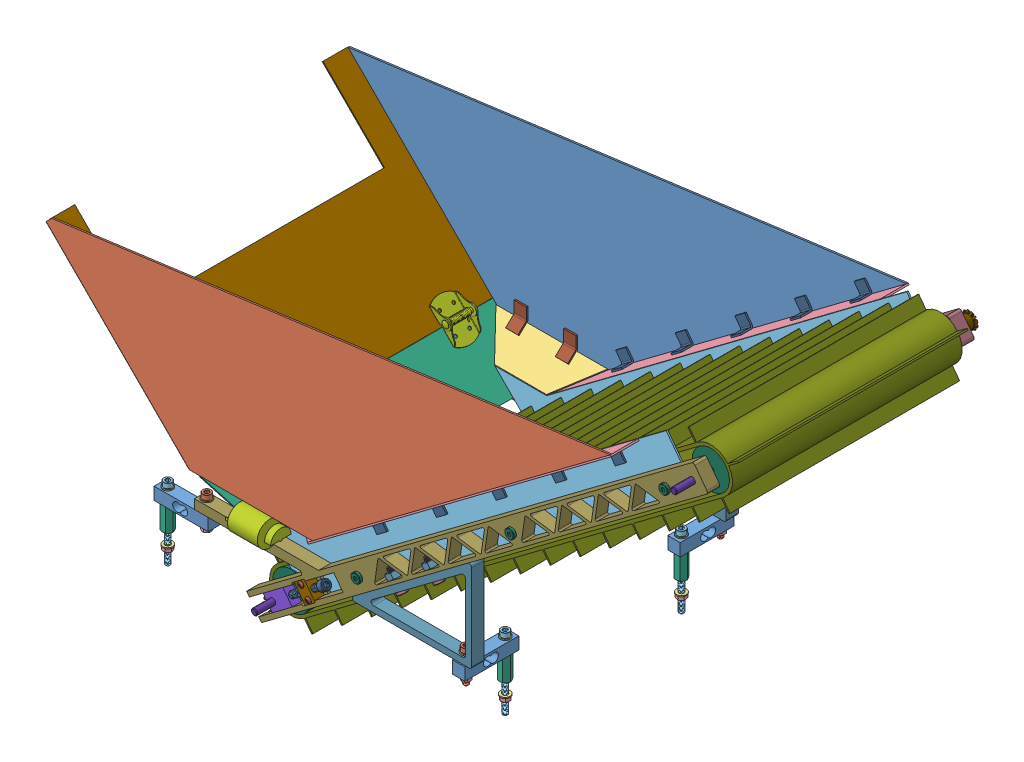
SolidWorks assembly Assembly_Hopper-Output, configuration Default. Lengths in mm.
Overall size (694.79 448.62 314.31).
124 component instances, 33 part files, 140 mates.
Components (placement in the parent):
- Side Plate Right-1: Side Plate Right [Default] at origin size (577.96 228.6 12.7)
- Side Plate Left-1: Side Plate Left [Default] at (0 0 303.2125) size (577.96 228.6 12.7)
- Slide-1: Slide [Default] at (0 1.1528 2.6789) x (1 0 0) z (0 -0.726184 -0.6875) size (114.3 38.1 1.59)
- Flap (Beside Conveyor)-4: Flap (Beside Conveyor) [Default] at (419.1 228.6 28.575) x (-0.8 -0.6 0) z (0.6 -0.8 0) size (425.45 28.57 1.59)
- Side Support-1: Side Support [Default] at (26.1937 -26.1937 28.575) size (451.96 314.33 1.59)
- Front Mesh 2-1: Front Mesh 2 [9227T543] at (20.048 -20.8922 152.4) x (0.707107 -0.707107 0) z (0 0 1) size (69.85 1.19 304.8)
- Front Hinge Bent-1: Front Hinge Bent [1613A11] at (-4.5491 4.5491 40.8686) x (0 0 -1) z (0.707107 -0.707107 0) size (30 12.7 42.82)
- Front Hinge Bent-4: Front Hinge Bent [1613A11] at (-7.2432 7.2432 264.7188) x (0 0 -1) z (0.707107 -0.707107 0) size (30 12.7 42.82)
- Front Folding Mesh-1: Front Folding Mesh [Default] at (-155.6871 149.5086 300.0375) x (-0.707107 -0.707107 0) z (0.707107 -0.707107 0) size (7.54 301.62 209.55)
  - Front Frame-1: Front Frame [Default] at origin size (6.35 301.62 209.55)
  - Front Mesh-1: Front Mesh [9227T543] at (-3.7719 147.6375 104.775) x (0 -1 0) z (0 0 1) size (301.62 1.19 209.55)
- Fastener-3: Fastener [Default] at (384.556 202.692 1.5875) x (0 0 1) z (-0.8 -0.6 0) size (12.7 12.7 12.7)
- Fastener-4: Fastener [Default] at (323.596 156.972 1.5875) x (0 0 1) z (-0.8 -0.6 0) size (12.7 12.7 12.7)
- Fastener-5: Fastener [Default] at (262.636 111.252 1.5875) x (0 0 1) z (-0.8 -0.6 0) size (12.7 12.7 12.7)
- Fastener-6: Fastener [Default] at (389.5725 204.47 28.575) x (0.6 -0.8 0) z (0.8 0.6 0) size (12.7 12.7 12.7)
- Fastener2-1: Fastener2 [Default] at (31.75 2.1861 1.5875) x (0 -0.6875 0.726184) z (-1 0 0) size (21.43 10.31 12.7)
- Fastener-7: Fastener [Default] at (328.6125 158.75 28.575) x (0.6 -0.8 0) z (0.8 0.6 0) size (12.7 12.7 12.7)
- Fastener-8: Fastener [Default] at (267.6525 113.03 28.575) x (0.6 -0.8 0) z (0.8 0.6 0) size (12.7 12.7 12.7)
- Fastener-10: Fastener [Default] at (374.396 195.072 303.2125) x (0 0 -1) z (0.8 0.6 0) size (12.7 12.7 12.7)
- Flap (Beside Conveyor)-5: Flap (Beside Conveyor) [Default] at (420.0525 227.33 276.225) x (-0.8 -0.6 0) z (-0.6 0.8 0) size (425.45 28.57 1.59)
- Fastener-13: Fastener [Default] at (313.436 149.352 303.2125) x (0 0 -1) z (0.8 0.6 0) size (12.7 12.7 12.7)
- Fastener-14: Fastener [Default] at (252.476 103.632 303.2125) x (0 0 -1) z (0.8 0.6 0) size (12.7 12.7 12.7)
- Slide-3: Slide [Default] at (0 0 303.2125) x (1 0 0) z (0 0.726184 -0.6875) size (114.3 38.1 1.59)
- Side Support-2: Side Support [Default] at (26.1937 -26.1937 274.6375) size (451.96 314.33 1.59)
- Fastener-16: Fastener [Default] at (399.7325 212.09 276.225) x (0.6 -0.8 0) z (-0.8 -0.6 0) size (12.7 12.7 12.7)
- Conveyor Beam Left-7: Conveyor Beam Left [Default] at (31.115 -94.1387 288.925) x (0.8 0.6 0) z (0 0 -1) size (586.74 101.6 12.7)
- Conveyor Beam Right-1: Conveyor Beam Right [Default] at (31.115 -94.1387 28.575) x (0.8 0.6 0) z (0 0 -1) size (586.74 101.6 12.7)
- Support-1: Support [Default] at (134.4083 -48.4188 276.225) size (121.92 92.72 12.7)
- Roller-1: Roller [Default] at (487.045 231.9338 34.925) x (-0.796427 -0.604735 0) z (0 0 1) size (38.1 38.1 234.95)
- Conveyor-1: Conveyor [Default] at (53.975 -116.6812 34.925) x (0.8 0.6 0) z (0 0 1) size (606.4 69.85 234.95)
- 12 inch shaft-1: 12 inch shaft [1257K66] at (487.045 231.9338 155.575) x (-0.158208 -0.987406 0) z (0 0 1) size (6.35 6.35 304.8)
- Gear2.0-1: Gear2.0 [6529K42] at (487.045 231.9338 15.0812) x (1 0 0) z (0 1 0) size (16.68 12.39 16.68)
- Roller-2: Roller [Default] at (57.785 -90.0113 269.875) x (0.803545 0.595244 0) z (0 0 -1) size (38.1 38.1 234.95)
- Fastener-17: Fastener [Default] at (338.7725 166.37 276.225) x (0.6 -0.8 0) z (-0.8 -0.6 0) size (12.7 12.7 12.7)
- Fastener-18: Fastener [Default] at (277.8125 120.65 276.225) x (0.6 -0.8 0) z (-0.8 -0.6 0) size (12.7 12.7 12.7)
- 12 inch shaft-2: 12 inch shaft [1257K66] at (57.785 -90.0113 155.575) x (0.992208 -0.124594 0) z (0 0 -1) size (6.35 6.35 304.8)
- Load_Cell_20_kg-1: Load_Cell_20_kg [Default] at (255.6933 -61.1187 290.195) x (0 0 -1) z (0 1 0) size (55.25 12.7 12.77)
- Load_Cell_20_kg-2: Load_Cell_20_kg [Default] at (242.9933 -61.1187 14.605) x (0 0 1) z (0 1 0) size (55.25 12.7 12.77)
- Load_Cell_20_kg-3: Load_Cell_20_kg [Default] at (-63.5 -61.1187 288.925) x (1 0 0) z (0 1 0) size (55.25 12.7 12.77)
- Load_Cell_20_kg-4: Load_Cell_20_kg [Default] at (-63.5 -61.1187 28.575) x (1 0 0) z (0 1 0) size (55.25 12.7 12.77)
- Screw for Load Cell M5x0.8x30mm-1: Screw for Load Cell M5x0.8x30mm [91290A194] at (-15.875 -50.2937 282.575) x (-0.988347 0 0.152214) z (0 1 0) size (8.5 8.5 35.43)
- Washer for Load Cell Screw-1: Washer for Load Cell Screw [93475A240] at (-15.875 -37.7938 282.575) x (1 0 0) z (0 -1 0) size (10 10 1.1)
- Washer for Load Cell Screw-2: Washer for Load Cell Screw [93475A240] at (-15.875 -62.2188 282.575) x (1 0 0) z (0 1 0) size (10 10 1.1)
- Nut for Load Cell Screw-2: Nut for Load Cell Screw [90592A095] at (-15.875 -64.2188 282.575) x (-0.979134 0 0.203217) z (-0.203217 0 -0.979134) size (8 4.62 9.24)
- Screw for Load Cell M5x0.8x30mm-2: Screw for Load Cell M5x0.8x30mm [91290A194] at (-15.875 -50.2937 22.225) x (-0.988347 0 -0.152214) z (0 1 0) size (8.5 8.5 35.43)
- Washer for Load Cell Screw-3: Washer for Load Cell Screw [93475A240] at (-15.875 -61.1187 22.225) x (1 0 0) z (0 -1 0) size (10 10 1.1)
- Washer for Load Cell Screw-4: Washer for Load Cell Screw [93475A240] at (-15.875 -38.8937 22.225) x (1 0 0) z (0 1 0) size (10 10 1.1)
- Screw for Load Cell M5x0.8x30mm-3: Screw for Load Cell M5x0.8x30mm [91290A194] at (249.3433 -53.4688 282.575) x (1 0 0) z (0 1 0) size (8.5 8.5 35.43)
- Washer for Load Cell Screw-5: Washer for Load Cell Screw [93475A240] at (249.3433 -40.9688 282.575) x (1 0 0) z (0 -1 0) size (10 10 1.1)
- Washer for Load Cell Screw-6: Washer for Load Cell Screw [93475A240] at (249.3433 -62.2188 282.575) x (1 0 0) z (0 1 0) size (10 10 1.1)
- Screw for Load Cell M5x0.8x30mm-4: Screw for Load Cell M5x0.8x30mm [91290A194] at (249.3433 -53.4688 22.225) x (1 0 0) z (0 1 0) size (8.5 8.5 35.43)
- Washer for Load Cell Screw-7: Washer for Load Cell Screw [93475A240] at (249.3433 -61.1187 22.225) x (1 0 0) z (0 -1 0) size (10 10 1.1)
- Washer for Load Cell Screw-8: Washer for Load Cell Screw [93475A240] at (249.3433 -42.0688 22.225) x (1 0 0) z (0 1 0) size (10 10 1.1)
- Nut for Load Cell Screw-1: Nut for Load Cell Screw [90592A095] at (249.3433 -64.2188 282.575) size (8 4.62 9.24)
- Screw for Load Cell M5x0.8x70mm-3: Screw for Load Cell M5x0.8x70mm [91290A201] at (249.3433 -79.8187 242.57) x (1 0 0) z (0 1 0) size (8.5 8.5 75.67)
- Load Cell Spacer-2: Load Cell Spacer [95947A747] at (249.3433 -86.1187 242.57) x (0 1 0) z (-0.546944 0 0.837169) size (25.61 10 11.55)
- Washer for Load Cell Screw-9: Washer for Load Cell Screw [93475A240] at (249.3433 -47.3188 242.57) x (1 0 0) z (0 -1 0) size (10 10 1.1)
- Washer for Load Cell Screw-17: Washer for Load Cell Screw [93475A240] at (249.3433 -99.9188 242.57) x (-0.837169 0 -0.546944) z (0 1 0) size (10 10 1.1)
- Nut for Load Cell Screw-7: Nut for Load Cell Screw [90592A095] at (249.3433 -101.9188 242.57) x (0.333464 0 0.942763) z (-0.942763 0 0.333464) size (8 4.62 9.24)
- Screw for Load Cell M5x0.8x70mm-1: Screw for Load Cell M5x0.8x70mm [91290A201] at (-55.88 -79.8187 282.575) x (1 0 0) z (0 1 0) size (8.5 8.5 75.67)
- Load Cell Spacer-1: Load Cell Spacer [95947A747] at (-55.88 -86.1187 282.575) x (0 1 0) z (0.546944 0 -0.837169) size (25.61 10 11.55)
- Washer for Load Cell Screw-10: Washer for Load Cell Screw [93475A240] at (-55.88 -48.4188 282.575) x (1 0 0) z (0 1 0) size (10 10 1.1)
- Washer for Load Cell Screw-14: Washer for Load Cell Screw [93475A240] at (-55.88 -98.8187 282.575) x (1 0 0) z (0 -1 0) size (10 10 1.1)
- Nut for Load Cell Screw-5: Nut for Load Cell Screw [90592A095] at (-55.88 -101.9188 282.575) x (-0.16458 0 0.986364) z (0.986364 0 0.16458) size (8 4.62 9.24)
- Washer for Load Cell Screw-11: Washer for Load Cell Screw [93475A240] at (-55.88 -47.3188 22.225) x (1 0 0) z (0 -1 0) size (10 10 1.1)
- Nut for Load Cell Screw-3: Nut for Load Cell Screw [90592A095] at (-15.875 -64.242 22.225) x (-0.979134 0 -0.203217) z (-0.203217 0 0.979134) size (8 4.62 9.24)
- Nut for Load Cell Screw-4: Nut for Load Cell Screw [90592A095] at (249.3433 -64.242 22.225) x (1 0 0) z (0 0 -1) size (8 4.62 9.24)
- Washer for Load Cell Screw-12: Washer for Load Cell Screw [93475A240] at (249.3433 -48.4188 62.23) x (1 0 0) z (0 1 0) size (10 10 1.1)
- Vibratory_Motor-1: Vibratory_Motor [Default] at (43.815 -26.9439 11.5748) x (0 0 -1) z (1 0 0) size (25.4 25.4 47.5)
- Vibratory_Motor-2: Vibratory_Motor [Default] at (43.815 -26.9439 293.2252) x (0 0 -1) z (1 0 0) size (25.4 25.4 47.5)
- Washer for Load Cell Screw-16: Washer for Load Cell Screw [93475A240] at (-55.88 -99.9188 22.225) x (1 0 0) z (0 1 0) size (10 10 1.1)
- Nut for Load Cell Screw-6: Nut for Load Cell Screw [90592A095] at (-55.88 -101.8955 22.225) x (-0.16458 0 -0.986364) z (0.986364 0 -0.16458) size (8 4.62 9.24)
- Washer for Load Cell Screw-19: Washer for Load Cell Screw [93475A240] at (249.3433 -98.8187 62.23) x (-0.837169 0 0.546944) z (0 -1 0) size (10 10 1.1)
- Nut for Load Cell Screw-8: Nut for Load Cell Screw [90592A095] at (249.3433 -101.942 62.23) x (0.333464 0 -0.942763) z (-0.942763 0 -0.333464) size (8 4.62 9.24)
- Fastener2-5: Fastener2 [Default] at (82.55 2.1861 1.5875) x (0 -0.6875 0.726184) z (-1 0 0) size (21.43 10.31 12.7)
- Fastener2-6: Fastener2 [Default] at (19.05 2.1861 303.2125) x (0 -0.6875 -0.726184) z (1 0 0) size (21.43 10.31 12.7)
- Fastener2-7: Fastener2 [Default] at (69.85 2.1861 303.2125) x (0 -0.6875 -0.726184) z (1 0 0) size (21.43 10.31 12.7)
- Fastener-21: Fastener [Default] at (201.676 65.532 1.5875) x (0 0 1) z (-0.8 -0.6 0) size (12.7 12.7 12.7)
- Fastener-22: Fastener [Default] at (140.716 19.812 1.5875) x (0 0 1) z (-0.8 -0.6 0) size (12.7 12.7 12.7)
- Fastener-24: Fastener [Default] at (191.516 57.912 303.2125) x (0 0 -1) z (0.8 0.6 0) size (12.7 12.7 12.7)
- Fastener-25: Fastener [Default] at (130.556 12.192 303.2125) x (0 0 -1) z (0.8 0.6 0) size (12.7 12.7 12.7)
- Fastener-27: Fastener [Default] at (206.6925 67.31 28.575) x (0.6 -0.8 0) z (0.8 0.6 0) size (12.7 12.7 12.7)
- Fastener-28: Fastener [Default] at (145.7325 21.59 28.575) x (0.6 -0.8 0) z (0.8 0.6 0) size (12.7 12.7 12.7)
- Fastener-30: Fastener [Default] at (216.8525 74.93 276.225) x (0.6 -0.8 0) z (-0.8 -0.6 0) size (12.7 12.7 12.7)
- Fastener-31: Fastener [Default] at (155.8925 29.21 276.225) x (0.6 -0.8 0) z (-0.8 -0.6 0) size (12.7 12.7 12.7)
- Hopper Tensioner A-2: Hopper Tensioner A [Default] at (79.6925 -87.4712 279.4) x (0 0 1) z (-0.8 -0.6 0) size (9.53 22.23 25.4)
- Hopper Tensioner B-1: Hopper Tensioner B [Default] at (91.186 -76.8667 278.765) x (0.8 0.6 0) z (0 0 1) size (12.74 19.05 10.16)
- Hopper tensioner bolt-1: Hopper tensioner bolt [90044A354] at (82.858 -71.2065 284.1625) x (-0.8 -0.6 0) z (-0.3 0.4 0.866025) size (57.82 9.53 9.53)
- hopper tensioner small bolt-1: hopper tensioner small bolt [92949A332] at (86.741 -60.3567 280.2382) size (6.05 6.05 21.13)
- hopper tensioner small bolt-2: hopper tensioner small bolt [92949A332] at (94.361 -70.5168 280.2382) size (6.05 6.05 21.13)
- hopper tensioner small nut-1: hopper tensioner small nut [90670A222] at (86.741 -60.3567 273.2484) x (0.99282 0.119615 0) z (0 0 1) size (7.94 9.17 3.16)
- hopper tensioner small nut-2: hopper tensioner small nut [90670A222] at (94.361 -70.5168 274.8359) x (0.39282 0.919615 0) z (0 0 1) size (7.94 9.17 3.16)
- Hopper Tensioner A-3: Hopper Tensioner A [Default] at (66.3575 -69.6912 25.4) x (0 0 -1) z (-0.8 -0.6 0) size (9.53 22.23 25.4)
- Hopper Tensioner B-2: Hopper Tensioner B [Default] at (91.186 -76.8667 15.875) x (0.8 0.6 0) z (0 0 1) size (12.74 19.05 10.16)
- hopper tensioner small bolt-3: hopper tensioner small bolt [92949A332] at (86.741 -60.3567 24.5618) x (1 0 0) z (0 0 -1) size (6.05 6.05 21.13)
- hopper tensioner small bolt-4: hopper tensioner small bolt [92949A332] at (94.361 -70.5168 24.5618) x (1 0 0) z (0 0 -1) size (6.05 6.05 21.13)
- Hopper tensioner bolt-2: Hopper tensioner bolt [90044A354] at (82.858 -71.2065 20.6375) x (-0.8 -0.6 0) z (-0.3 0.4 -0.866025) size (57.82 9.53 9.53)
- hopper tensioner small nut-3: hopper tensioner small nut [90670A222] at (94.361 -70.5168 30.0924) x (0.39282 0.919615 0) z (0 0 1) size (7.94 9.17 3.16)
- hopper tensioner small nut-4: hopper tensioner small nut [90670A222] at (86.741 -60.3567 31.6799) x (0.99282 0.119615 0) z (0 0 1) size (7.94 9.17 3.16)
- Support-3: Support [Default] at (134.4083 -48.4188 15.875) size (121.92 92.72 12.7)
- Load Cell Spacer-3: Load Cell Spacer [95947A747] at (-55.88 -86.1187 22.225) x (0 1 0) z (-0.546944 0 -0.837169) size (25.61 10 11.55)
- Screw for Load Cell M5x0.8x70mm-2: Screw for Load Cell M5x0.8x70mm [91290A201] at (-55.88 -79.8187 22.225) x (1 0 0) z (0 1 0) size (8.5 8.5 75.67)
- Load Cell Spacer-4: Load Cell Spacer [95947A747] at (249.3433 -61.0961 62.23) x (0 -1 0) z (0.546944 0 0.837169) size (25.61 10 11.55)
- Screw for Load Cell M5x0.8x70mm-4: Screw for Load Cell M5x0.8x70mm [91290A201] at (249.3433 -79.8187 62.23) x (1 0 0) z (0 1 0) size (8.5 8.5 75.67)
- Conveyor beam 0.75 in screw-1: Conveyor beam 0.75 in screw [93615A415] at (209.0022 23.4016 282.575) x (0.64 0.48 0.6) z (-0.6 0.8 0) size (9.53 9.53 22.88)
- Conveyor beam 0.75 in screw-2: Conveyor beam 0.75 in screw [93615A415] at (171.4102 -4.7924 282.575) x (0.64 0.48 0.6) z (-0.6 0.8 0) size (9.53 9.53 22.88)
- Conveyor Beam nut-1: Conveyor Beam nut [95505A601] at (175.4583 -10.1899 282.575) x (-0.64 -0.48 0.6) z (0.6 -0.8 0) size (11.11 12.83 6.51)
- Conveyor Beam nut-2: Conveyor Beam nut [95505A601] at (213.0503 18.0041 282.575) x (-0.64 -0.48 0.6) z (0.6 -0.8 0) size (11.11 12.83 6.51)
- Conveyor beam 0.75 in screw-3: Conveyor beam 0.75 in screw [93615A415] at (171.4102 -4.7924 22.225) x (-0.64 -0.48 0.6) z (-0.6 0.8 0) size (9.53 9.53 22.88)
- Conveyor Beam nut-3: Conveyor Beam nut [95505A601] at (175.4589 -10.1907 22.225) x (0.64 0.48 0.6) z (-0.6 0.8 0) size (11.11 12.83 6.51)
- Conveyor beam 0.75 in screw-4: Conveyor beam 0.75 in screw [93615A415] at (209.0022 23.4016 22.225) x (-0.64 -0.48 0.6) z (-0.6 0.8 0) size (9.53 9.53 22.88)
- Conveyor Beam nut-4: Conveyor Beam nut [95505A601] at (213.0509 18.0033 22.225) x (0.64 0.48 0.6) z (-0.6 0.8 0) size (11.11 12.83 6.51)
- conveyor beam 1.0 in screw-1: conveyor beam 1.0 in screw [93615A420] at (145.415 -24.2888 263.525) x (-0.923728 -0.383049 0) z (0 0 -1) size (9.53 9.53 29.27)
- conveyor beam 1.0 in screw-2: conveyor beam 1.0 in screw [93615A420] at (460.375 211.9312 263.525) x (-0.923728 -0.383049 0) z (0 0 -1) size (9.53 9.53 29.27)
- conveyor beam 1.0 in screw-3: conveyor beam 1.0 in screw [93615A420] at (302.895 93.8212 263.525) x (-0.923728 -0.383049 0) z (0 0 -1) size (9.53 9.53 29.27)
- Conveyor Beam nut-5: Conveyor Beam nut [95505A601] at (302.895 93.8212 271.8594) x (-0.706547 -0.707666 0) z (0 0 1) size (11.11 12.83 6.51)
- Conveyor Beam nut-6: Conveyor Beam nut [95505A601] at (460.375 211.9312 271.8594) x (0.706547 0.707666 0) z (0 0 -1) size (11.11 12.83 6.51)
- Conveyor Beam nut-7: Conveyor Beam nut [95505A601] at (145.415 -24.2888 271.8594) x (-0.923728 -0.383049 0) z (0 0 1) size (11.11 12.83 6.51)
- conveyor beam 1.0 in screw-4: conveyor beam 1.0 in screw [93615A420] at (460.375 211.9312 41.275) x (-0.923728 -0.383049 0) z (0 0 1) size (9.53 9.53 29.27)
- Conveyor Beam nut-8: Conveyor Beam nut [95505A601] at (460.375 211.9312 32.9416) x (-0.706547 -0.707666 0) z (0 0 -1) size (11.11 12.83 6.51)
- conveyor beam 1.0 in screw-5: conveyor beam 1.0 in screw [93615A420] at (302.895 93.8212 41.275) x (-0.923728 -0.383049 0) z (0 0 1) size (9.53 9.53 29.27)
- Conveyor Beam nut-9: Conveyor Beam nut [95505A601] at (302.895 93.8212 32.9396) x (-0.706547 -0.707666 0) z (0 0 1) size (11.11 12.83 6.51)
- conveyor beam 1.0 in screw-6: conveyor beam 1.0 in screw [93615A420] at (145.415 -24.2888 41.275) x (-0.923728 -0.383049 0) z (0 0 1) size (9.53 9.53 29.27)
- Conveyor Beam nut-10: Conveyor Beam nut [95505A601] at (145.415 -24.2888 32.9396) x (-0.923728 -0.383049 0) z (0 0 1) size (11.11 12.83 6.51)
Mates (geometry in assembly coordinates):
- Coincident4: coincident aligned: line of Slide-1 through (0 0 1.5875) axis (1 0 0); line of Side Plate-1 through (-10.6685 0 1.5875) axis (1 0 0)
- Coincident19: coincident anti-aligned: line of Side Plate-1 through (419.1 228.6 1.5875) axis (0 0 -1); line of Flap (Beside Conveyor)-4 through (419.1 228.6 0) axis (0 0 1)
- Coincident21: coincident aligned: line of Side Support-1 through (447.675 250.0312 28.575) axis (-0.8 -0.6 0); line of Flap (Beside Conveyor)-4 through (419.1 228.6 28.575) axis (-0.8 -0.6 0)
- Coincident27: coincident anti-aligned: plane of Side Plate-1 through (0 0 1.5875) normal (0 0 1); plane of Fastener-3 through (366.776 205.232 1.5875) normal (0 0 -1)
- Coincident28: coincident anti-aligned: plane of Flap (Beside Conveyor)-4 through (419.1 228.6 28.575) normal (-0.6 0.8 0); plane of Fastener-3 through (374.396 195.072 4.1275) normal (0.6 -0.8 0)
- Distance2: distance = 43.18 mm: plane of Fastener-3 through (382.8415 204.978 4.445) normal (0.8 0.6 0); line of Flap (Beside Conveyor)-4 through (419.1 228.6 0) axis (0 0 1)
- Coincident30: coincident anti-aligned: plane of Side Support-1 through (26.1937 -26.1937 28.575) normal (0 0 -1); plane of Fastener-6 through (401.2565 210.058 28.575) normal (0 0 1)
- Coincident31: coincident anti-aligned: plane of Flap (Beside Conveyor)-4 through (420.0525 227.33 28.575) normal (0.6 -0.8 0); plane of Fastener-6 through (399.7325 212.09 15.875) normal (-0.6 0.8 0)
- Distance3: distance = 25.4 mm aligned: plane of Fastener-6 through (401.447 209.804 25.7175) normal (0.8 0.6 0); plane of Flap (Beside Conveyor)-4 through (420.0525 227.33 0) normal (0.8 0.6 0)
- Coincident66: coincident anti-aligned: plane of Side Support-2 through (26.1937 -26.1937 276.225) normal (0 0 1); plane of Conveyor Beam-7 through (499.999 228.9493 276.225) normal (0 0 -1)
- Distance25: distance = 117.475 mm aligned: plane of Roller-1 through (487.045 231.9338 269.875) normal (0 0 1)
- Concentric8: concentric aligned: cylinder of Roller-1 through (487.045 231.9338 269.875) axis (0 0 -1) radius 19.05; cylinder of Conveyor-1 through (487.045 231.9338 269.875) axis (0 0 -1) radius 19.05
- Coincident81: coincident aligned: plane of Roller-1 through (487.045 231.9338 269.875) normal (0 0 1); plane of Conveyor-1 through (57.785 -90.0112 269.875) normal (0 0 1)
- Coincident83: coincident anti-aligned: plane of Conveyor Beam-7 through (501.523 226.9172 276.225) normal (0.6 -0.8 0); plane of Support-1 through (257.3443 43.7833 288.925) normal (-0.6 0.8 0)
- Coincident124: coincident aligned: plane of Conveyor Beam-7 through (-22.225 -48.4188 276.225) normal (0 -1 0); plane of Support-1 through (142.0283 -48.4188 288.925) normal (0 -1 0)
- Coincident120: coincident aligned: line of Conveyor Beam-7 through (501.523 226.9172 288.925) axis (-0.8 -0.6 0); line of Support-1 through (257.3443 43.7833 288.925) axis (-0.8 -0.6 0)
- Distance45: distance = 27.051 mm: line of Front Mesh 2-1 through (45.1658 -45.1658 279.4) axis (0 0 -1); line of Side Support-1 through (64.2938 -64.2938 30.1625) axis (0 0 -1)
- Coincident109: coincident: point of Side Plate-1; point of Flap (Beside Conveyor)-4
- Concentric13: concentric aligned: cylinder of Roller-1 through (487.045 231.9338 269.875) axis (0 0 -1) radius 3.175; cylinder of 12 inch shaft-1 through (487.045 231.9338 307.975) axis (0 0 -1) radius 3.175
- Concentric15: concentric aligned: cylinder of Gear2.0-1 through (487.045 231.9338 -1.985) axis (0 0 -1) radius 3.175; cylinder of 12 inch shaft-1 through (487.045 231.9338 307.975) axis (0 0 -1) radius 3.175
- Coincident118: coincident: line of Slide-1 through (79.375 -26.1937 29.2551) axis (-1 0 0); plane of Side Support-1 through (26.1937 -26.1937 30.1625) normal (0 1 0)
- Parallel4: parallel aligned: line of Side Support-1 through (447.675 250.0312 28.575) axis (-0.8 -0.6 0); line of Conveyor-1 through (475.615 247.1737 34.925) axis (-0.8 -0.6 0)
- Coincident121: coincident anti-aligned: plane of Support-1 through (142.0283 -48.4188 288.925) normal (0 -1 0); plane of Load_Cell_20_kg-1 through (255.6933 -48.4188 290.195) normal (0 1 0)
- Coincident125: coincident anti-aligned: plane of Conveyor Beam-7 through (-22.225 -48.4188 276.225) normal (0 -1 0); plane of Load_Cell_20_kg-3 through (-63.5 -48.4188 288.925) normal (0 1 0)
- Coincident126: coincident anti-aligned: line of Conveyor Beam-7 through (85.725 -48.4188 288.925) axis (-1 0 0); line of Load_Cell_20_kg-3 through (-63.5 -48.4188 288.925) axis (1 0 0)
- Concentric18: concentric anti-aligned: circle of Support-1; circle of Load_Cell_20_kg-1
- Parallel5: parallel aligned: line of Support-1 through (142.0283 -48.4188 288.925) axis (1 0 0); line of Load_Cell_20_kg-1 through (242.9933 -48.4188 290.195) axis (1 0 0)
- Coincident135: coincident anti-aligned: plane of Load_Cell_20_kg-4 through (-63.5 -48.4188 28.575) normal (0 1 0); plane of Conveyor Beam Right-1 through (-22.225 -48.4188 15.875) normal (0 -1 0)
- Coincident136: coincident anti-aligned: plane of Side Support-1 through (26.1937 -26.1937 28.575) normal (0 0 -1); plane of Conveyor Beam Right-1 through (499.999 228.9493 28.575) normal (0 0 1)
- Coincident137: coincident anti-aligned: circle of Conveyor Beam-7; circle of Load_Cell_20_kg-3
- Concentric21: concentric anti-aligned: circle of Load_Cell_20_kg-3; circle of Screw for Load Cell M5x0.8x30mm-1
- Coincident138: coincident anti-aligned: plane of Conveyor Beam-7 through (104.775 -38.8937 276.225) normal (0 1 0); plane of Washer for Load Cell Screw-1 through (-15.875 -38.8937 282.575) normal (0 -1 0)
- Concentric22: concentric anti-aligned: circle of Load_Cell_20_kg-3; circle of Washer for Load Cell Screw-1
- Coincident139: coincident anti-aligned: plane of Screw for Load Cell M5x0.8x30mm-1 through (-11.9216 -37.7938 281.9661) normal (0 -1 0); plane of Washer for Load Cell Screw-1 through (-15.875 -37.7938 282.575) normal (0 1 0)
- Coincident140: coincident anti-aligned: plane of Load_Cell_20_kg-3 through (-63.5 -61.1187 288.925) normal (0 -1 0); plane of Washer for Load Cell Screw-2 through (-15.875 -61.1187 282.575) normal (0 1 0)
- Concentric23: concentric aligned: circle of Load_Cell_20_kg-3; circle of Washer for Load Cell Screw-2
- Coincident141: coincident anti-aligned: plane of Support-1 through (161.0783 -42.0688 288.925) normal (0 1 0); plane of Washer for Load Cell Screw-5 through (249.3433 -42.0688 282.575) normal (0 -1 0)
- Concentric24: concentric anti-aligned: circle of Load_Cell_20_kg-1; circle of Washer for Load Cell Screw-5
- Coincident142: coincident anti-aligned: plane of Screw for Load Cell M5x0.8x30mm-3 through (245.3433 -40.9688 282.575) normal (0 -1 0); plane of Washer for Load Cell Screw-5 through (249.3433 -40.9688 282.575) normal (0 1 0)
- Concentric25: concentric anti-aligned: circle of Load_Cell_20_kg-1; circle of Screw for Load Cell M5x0.8x30mm-3
- Coincident143: coincident anti-aligned: plane of Load_Cell_20_kg-1 through (255.6933 -61.1187 290.195) normal (0 -1 0); plane of Washer for Load Cell Screw-6 through (249.3433 -61.1187 282.575) normal (0 1 0)
- Concentric26: concentric aligned: circle of Load_Cell_20_kg-1; circle of Washer for Load Cell Screw-6
- Coincident144: coincident anti-aligned: plane of Washer for Load Cell Screw-6 through (249.3433 -62.2188 282.575) normal (0 -1 0); plane of Nut for Load Cell Screw-1 through (245.3433 -62.2188 280.2656) normal (0 1 0)
- Concentric27: concentric aligned: circle of Washer for Load Cell Screw-6; circle of Nut for Load Cell Screw-1
- Coincident145: coincident anti-aligned: plane of Washer for Load Cell Screw-2 through (-15.875 -62.2188 282.575) normal (0 -1 0); plane of Nut for Load Cell Screw-2 through (-11.4892 -62.2188 284.0233) normal (0 1 0)
- Concentric28: concentric aligned: circle of Washer for Load Cell Screw-2; circle of Nut for Load Cell Screw-2
- Coincident149: coincident anti-aligned: plane of Load_Cell_20_kg-1 through (255.6933 -48.4188 290.195) normal (0 1 0); plane of Washer for Load Cell Screw-9 through (249.3433 -48.4188 242.57) normal (0 -1 0)
- Concentric29: concentric anti-aligned: circle of Load_Cell_20_kg-1; circle of Washer for Load Cell Screw-9
- Coincident151: coincident anti-aligned: plane of Load_Cell_20_kg-3 through (-63.5 -48.4188 288.925) normal (0 1 0); plane of Washer for Load Cell Screw-10 through (-55.88 -48.4188 282.575) normal (0 -1 0)
- Concentric31: concentric aligned: circle of Load_Cell_20_kg-3; circle of Washer for Load Cell Screw-10
- Coincident154: coincident: line of Conveyor Beam Right-1 through (-22.225 -38.8937 15.875) axis (1 0 0); cylinder of Vibratory_Motor-1 through (59.055 -26.9439 11.5748) axis (-1 0 0) radius 12.7
- Distance36: distance = 50.8 mm aligned: plane of Vibratory_Motor-1 through (28.575 -26.9439 11.5748) normal (-1 0 0); plane of Conveyor Beam Right-1 through (-22.225 -38.8937 15.875) normal (-1 0 0)
- Parallel6: parallel anti-aligned: plane of Conveyor Beam Right-1 through (104.775 -38.8937 15.875) normal (0 1 0); plane of Vibratory_Motor-1 through (64.135 -26.9439 22.0523) normal (0 -1 0)
- Coincident160: coincident anti-aligned: plane of Washer for Load Cell Screw-14 through (-55.88 -99.9188 282.575) normal (0 -1 0); plane of Nut for Load Cell Screw-5 through (-57.4996 -99.9188 278.2495) normal (0 1 0)
- Distance42: distance = 12.7 mm aligned: plane of 12 inch shaft-1 through (487.045 231.9338 3.175) normal (0 0 -1); plane of Conveyor Beam Right-1 through (499.999 228.9493 15.875) normal (0 0 -1)
- Coincident175: coincident: line of Slide-1 through (114.3 0 1.5875) axis (-0.675725 -0.506793 0.53531); plane of Flap (Beside Conveyor)-4 through (419.1 228.6 28.575) normal (-0.6 0.8 0)
- Distance43: distance = 31.75 mm: line of Conveyor Beam-7 through (489.839 246.7293 276.225) axis (0.6 -0.8 0); line of Side Support-2 through (478.155 209.3913 276.225) axis (-0.6 0.8 0)
- Tangent1: tangent anti-aligned: plane of Slide-1 through (0 0 1.5875) normal (0 -0.726184 -0.6875); cylinder of Vibratory_Motor-1 through (59.055 -26.9439 11.5748) axis (-1 0 0) radius 12.7
- Coincident176: coincident anti-aligned: plane of Side Plate-1 through (0 0 1.5875) normal (0 0 1); plane of Fastener2-1 through (19.05 14.8861 1.5875) normal (0 0 -1)
- Coincident179: coincident: plane of Slide-1 through (0 1.1528 2.6789) normal (0 0.726184 0.6875); line of Fastener2-1 through (19.05 -6.5452 10.81) axis (1 0 0)
- Distance44: distance = 19.05 mm: plane of Fastener2-1 through (19.05 3.9623 5.715) normal (-1 0 0); point of Slide-1
- Coincident184: coincident: plane of Front Mesh 2-1 through (45.1658 -45.1658 304.8) normal (0.707107 0.707107 0); line of Slide-3 through (26.1937 -26.1937 275.5449) axis (-0.566529 0.566529 0.598406)
- Coincident185: coincident: line of Slide-1 through (26.1937 -26.1937 29.2551) axis (-0.566529 0.566529 -0.598406); plane of Front Mesh 2-1 through (45.1658 -45.1658 304.8) normal (0.707107 0.707107 0)
- Coincident186: coincident anti-aligned: plane of Flap (Beside Conveyor)-5 through (419.1 228.6 276.225) normal (-0.6 0.8 0); plane of Side Plate Left-1 through (114.3 0 304.8) normal (0.6 -0.8 0)
- Coincident187: coincident aligned: line of Flap (Beside Conveyor)-5 through (419.1 228.6 304.8) axis (0 0 -1); line of Side Plate Left-1 through (419.1 228.6 304.8) axis (0 0 -1)
- Coincident188: coincident anti-aligned: plane of Fastener-10 through (376.936 212.852 303.2125) normal (0 0 1); plane of Side Plate Left-1 through (0 0 303.2125) normal (0 0 -1)
- Coincident189: coincident: plane of Side Plate-1 through (0 0 0) normal (0 0 -1); point of Front Mesh 2-1
- Tangent3: tangent anti-aligned: plane of Side Plate-1 through (0 0 1.5875) normal (0 0 1); cylinder of Front Folding Mesh-1/Front Frame-1 through (-7.5128 1.3344 4.7625) axis (-0.707107 0.707107 0) radius 3.175
- Parallel8: parallel anti-aligned: line of Front Folding Mesh-1/Front Mesh-1 through (-4.4236 4.4236 1.5875) axis (0 0 1); line of Front Hinge Bent-1 through (-2.3218 3.4353 52.6669) axis (0 0 -1)
- Coincident196: coincident anti-aligned: plane of Front Mesh 2-1 through (45.1658 -45.1658 304.8) normal (0.707107 0.707107 0); plane of Front Folding Mesh-1/Front Hinge-1 through (-3.8954 3.8954 39.1795) normal (-0.707107 -0.707107 0)
- Coincident197: coincident anti-aligned: plane of Front Mesh 2-1 through (45.1658 -45.1658 304.8) normal (0.707107 0.707107 0); plane of Front Folding Mesh-1/Front Hinge-2 through (-3.8954 3.8954 39.1795) normal (-0.707107 -0.707107 0)
- Coincident199: coincident anti-aligned: plane of Front Mesh 2-1 through (45.1658 -45.1658 304.8) normal (0.707107 0.707107 0); plane of Front Hinge Bent-1 through (-4.9336 4.9336 40.4749) normal (-0.707107 -0.707107 0)
- Parallel10: parallel anti-aligned: line of Front Mesh 2-1 through (-4.2256 4.2256 304.8) axis (0 0 -1); line of Front Folding Mesh-1/Front Mesh-1 through (-4.4236 4.4236 1.5875) axis (0 0 1)
- Coincident203: coincident anti-aligned: plane of Front Hinge Bent-1 through (-4.1647 4.1647 41.2623) normal (-0.707107 -0.707107 0); plane of Front Folding Mesh-1/Front Mesh-1 through (-4.4236 4.4236 303.2125) normal (0.707107 0.707107 0)
- Distance50: distance = 2.54 mm: line of Front Folding Mesh-1/Front Mesh-1 through (-4.4236 4.4236 1.5875) axis (0 0 1); line of Front Hinge Bent-1 through (-6.2197 6.2197 53.4543) axis (0 0 -1)
- Distance51: distance = 25.4 mm anti-aligned: plane of Side Plate-1 through (0 0 1.5875) normal (0 0 1); plane of Front Hinge Bent-1 through (0.6415 9.7397 26.9875) normal (0 0 -1)
- Coincident207: coincident anti-aligned: plane of Front Folding Mesh-1/Front Mesh-1 through (-4.4236 4.4236 303.2125) normal (0.707107 0.707107 0); plane of Front Hinge Bent-4 through (-6.8588 6.8588 265.1125) normal (-0.707107 -0.707107 0)
- Parallel11: parallel anti-aligned: line of Front Hinge Bent-4 through (-8.9137 8.9137 277.3045) axis (0 0 -1); line of Front Folding Mesh-1/Front Mesh-1 through (-4.4236 4.4236 1.5875) axis (0 0 1)
- Distance54: distance = 6.35 mm: line of Front Hinge Bent-4 through (-8.9137 8.9137 277.3045) axis (0 0 -1); line of Front Folding Mesh-1/Front Mesh-1 through (-4.4236 4.4236 1.5875) axis (0 0 1)
- Distance55: distance = 25.4 mm anti-aligned: plane of Side Plate Left-1 through (0 0 303.2125) normal (0 0 -1); plane of Front Hinge Bent-4 through (-2.0526 12.4338 277.8125) normal (0 0 1)
- Distance56: distance = 1.905 mm: line of Front Mesh 2-1 through (-4.2256 4.2256 304.8) axis (0 0 -1); line of Front Hinge Bent-1 through (-2.8786 2.8786 52.6669) axis (0 0 -1)
- Coincident210: coincident anti-aligned: plane of Conveyor Beam-7 through (80.9625 -86.5188 279.4) normal (0 0 1); plane of Hopper Tensioner A-2 through (46.0375 -84.9313 279.4) normal (0 0 -1)
- Coincident211: coincident anti-aligned: plane of Conveyor Beam-7 through (80.9625 -86.5188 282.575) normal (-0.6 0.8 0); plane of Hopper Tensioner A-2 through (59.3725 -102.7113 279.4) normal (0.6 -0.8 0)
- Coincident212: coincident anti-aligned: plane of Conveyor Beam-7 through (89.154 -78.3907 278.765) normal (-0.6 0.8 0); plane of Hopper Tensioner B-1 through (91.186 -76.8667 288.925) normal (0.6 -0.8 0)
- Coincident213: coincident: line of Conveyor Beam-7 through (101.346 -69.2467 278.765) axis (-0.8 -0.6 0); point of Hopper Tensioner B-1
- Coincident214: coincident anti-aligned: line of Conveyor Beam-7 through (101.346 -69.2467 278.765) axis (0 0 1); line of Hopper Tensioner B-1 through (101.346 -69.2467 288.925) axis (0 0 -1)
- Coincident215: coincident aligned: cone of Hopper Tensioner A-2 through (62.865 -86.2012 284.1625) axis (-0.8 -0.6 0); circle of Hopper tensioner bolt-1
- Parallel12: parallel aligned: plane of Conveyor Beam-7 through (100.3935 -67.9767 278.765) normal (-0.6 0.8 0); plane of Hopper tensioner bolt-1 through (107.2483 -55.8903 282.7877) normal (-0.6 0.8 0)
- Concentric57: concentric aligned: circle of Hopper Tensioner B-1; circle of hopper tensioner small bolt-2
- Coincident219: coincident anti-aligned: plane of Hopper Tensioner B-1 through (91.186 -76.8667 288.925) normal (0 0 1); plane of hopper tensioner small bolt-2 through (94.361 -67.4942 288.925) normal (0 0 -1)
- Concentric58: concentric aligned: circle of Hopper Tensioner B-1; circle of hopper tensioner small bolt-1
- Coincident220: coincident anti-aligned: plane of Hopper Tensioner B-1 through (91.186 -76.8667 288.925) normal (0 0 1); plane of hopper tensioner small bolt-1 through (86.741 -57.3342 288.925) normal (0 0 -1)
- Concentric59: concentric aligned: circle of hopper tensioner small bolt-2; circle of hopper tensioner small nut-2
- Coincident221: coincident anti-aligned: plane of Conveyor Beam-7 through (499.999 228.9493 276.225) normal (0 0 -1); plane of hopper tensioner small nut-2 through (90.6948 -73.2664 276.225) normal (0 0 1)
- Parallel13: parallel aligned: plane of Conveyor Beam-7 through (501.523 226.9172 276.225) normal (0.6 -0.8 0); plane of hopper tensioner small nut-2 through (94.9092 -75.0666 276.225) normal (0.6 -0.8 0)
- Concentric60: concentric aligned: circle of hopper tensioner small bolt-1; circle of hopper tensioner small nut-1
- Coincident223: coincident anti-aligned: plane of Side Support-2 through (26.1937 -26.1937 274.6375) normal (0 0 -1); plane of hopper tensioner small nut-1 through (82.5267 -58.5566 274.6375) normal (0 0 1)
- Parallel14: parallel aligned: plane of Conveyor Beam-7 through (501.523 226.9172 276.225) normal (0.6 -0.8 0); plane of hopper tensioner small nut-1 through (87.2892 -64.9066 274.6375) normal (0.6 -0.8 0)
- Distance57: distance = 25.4 mm: line of Side Support-2 through (447.675 250.0312 276.225) axis (-0.8 -0.6 0); line of Conveyor Beam-7 through (104.775 -38.8937 276.225) axis (0.8 0.6 0)
- Concentric61: concentric aligned: cylinder of Conveyor Beam Right-1 through (487.045 231.9338 15.875) axis (0 0 -1) radius 3.175; cylinder of 12 inch shaft-1 through (487.045 231.9338 307.975) axis (0 0 -1) radius 3.175
- Concentric63: concentric anti-aligned: cylinder of Conveyor Beam-7 through (487.045 231.9338 276.225) axis (0 0 1) radius 3.175; cylinder of 12 inch shaft-1 through (487.045 231.9338 307.975) axis (0 0 -1) radius 3.175
- Concentric64: concentric aligned: cylinder of 12 inch shaft-2 through (57.785 -90.0113 3.175) axis (0 0 1) radius 3.175; cylinder of Hopper Tensioner A-2 through (57.785 -90.0113 279.4) axis (0 0 1) radius 3.175
- Coincident227: coincident anti-aligned: plane of Washer for Load Cell Screw-10 through (-55.88 -47.3188 282.575) normal (0 1 0); plane of Screw for Load Cell M5x0.8x70mm-1 through (-59.88 -47.3188 282.575) normal (0 -1 0)
- Concentric66: concentric anti-aligned: circle of Washer for Load Cell Screw-10; circle of Screw for Load Cell M5x0.8x70mm-1
- Concentric67: concentric aligned: circle of Washer for Load Cell Screw-14; circle of Screw for Load Cell M5x0.8x70mm-1
- Concentric68: concentric anti-aligned: circle of Load_Cell_20_kg-3; circle of Screw for Load Cell M5x0.8x70mm-1
- Concentric69: concentric aligned: circle of Nut for Load Cell Screw-5; circle of Screw for Load Cell M5x0.8x70mm-1
- Coincident229: coincident anti-aligned: plane of Load_Cell_20_kg-3 through (-63.5 -61.1187 288.925) normal (0 -1 0); plane of Load Cell Spacer-1 through (-55.88 -61.1187 282.575) normal (0 1 0)
- Concentric70: concentric aligned: circle of Load Cell Spacer-1; circle of Screw for Load Cell M5x0.8x70mm-1
- Distance59: distance = 12.7 mm anti-aligned: plane of Load Cell Spacer-1 through (-55.88 -86.1187 282.575) normal (0 -1 0); plane of Washer for Load Cell Screw-14 through (-55.88 -98.8187 282.575) normal (0 1 0)
- Coincident231: coincident anti-aligned: plane of Washer for Load Cell Screw-9 through (249.3433 -47.3188 242.57) normal (0 1 0); plane of Screw for Load Cell M5x0.8x70mm-3 through (245.3433 -47.3188 242.57) normal (0 -1 0)
- Concentric71: concentric aligned: circle of Washer for Load Cell Screw-9; circle of Screw for Load Cell M5x0.8x70mm-3
- Concentric72: concentric anti-aligned: circle of Load_Cell_20_kg-1; circle of Screw for Load Cell M5x0.8x70mm-3
- Concentric73: concentric anti-aligned: circle of Nut for Load Cell Screw-7; circle of Screw for Load Cell M5x0.8x70mm-3
- Coincident233: coincident anti-aligned: plane of Load_Cell_20_kg-1 through (255.6933 -61.1187 290.195) normal (0 -1 0); plane of Load Cell Spacer-2 through (249.3433 -61.1187 242.57) normal (0 1 0)
- Concentric74: concentric aligned: circle of Load Cell Spacer-2; circle of Screw for Load Cell M5x0.8x70mm-3
- Coincident235: coincident anti-aligned: plane of Washer for Load Cell Screw-17 through (249.3433 -99.9188 242.57) normal (0 -1 0); plane of Nut for Load Cell Screw-7 through (250.1867 -99.9188 238.0288) normal (0 1 0)
- Distance61: distance = 12.7 mm anti-aligned: plane of Washer for Load Cell Screw-17 through (249.3433 -98.8187 242.57) normal (0 1 0); plane of Load Cell Spacer-2 through (249.3433 -86.1187 242.57) normal (0 -1 0)
- Concentric75: concentric anti-aligned: circle of Washer for Load Cell Screw-17; circle of Screw for Load Cell M5x0.8x70mm-3
- Concentric76: concentric anti-aligned: circle of Screw for Load Cell M5x0.8x70mm-3; circle of Nut for Load Cell Screw-7
- Coincident236: coincident anti-aligned: plane of Support-1 through (250.9943 31.0832 288.925) normal (0.6 -0.8 0); plane of Conveyor beam 0.75 in screw-2 through (182.8402 -20.0324 282.575) normal (-0.6 0.8 0)
- Concentric77: concentric anti-aligned: circle of Support-1; circle of Conveyor beam 0.75 in screw-2
- Coincident237: coincident anti-aligned: plane of Conveyor Beam-7 through (164.2508 -22.0681 276.225) normal (-0.6 0.8 0); plane of Conveyor Beam nut-1 through (179.1414 -10.9002 276.6749) normal (0.6 -0.8 0)
- Concentric78: concentric aligned: circle of Conveyor beam 0.75 in screw-2; circle of Conveyor Beam nut-1
- Coincident238: coincident anti-aligned: plane of Support-1 through (250.9943 31.0832 288.925) normal (0.6 -0.8 0); plane of Conveyor beam 0.75 in screw-1 through (220.4322 8.1616 282.575) normal (-0.6 0.8 0)
- Concentric79: concentric anti-aligned: circle of Support-1; circle of Conveyor beam 0.75 in screw-1
- Coincident239: coincident anti-aligned: plane of Conveyor Beam-7 through (201.8428 6.1259 276.225) normal (-0.6 0.8 0); plane of Conveyor Beam nut-2 through (216.7334 17.2938 276.6749) normal (0.6 -0.8 0)
- Concentric80: concentric aligned: circle of Conveyor beam 0.75 in screw-1; circle of Conveyor Beam nut-2
- Coincident240: coincident anti-aligned: plane of Conveyor Beam-7 through (499.999 228.9493 288.925) normal (0 0 1); plane of conveyor beam 1.0 in screw-2 through (460.375 211.9312 288.925) normal (0 0 -1)
- Concentric81: concentric anti-aligned: circle of Conveyor Beam-7; circle of conveyor beam 1.0 in screw-2
- Coincident241: coincident anti-aligned: plane of Conveyor Beam-7 through (499.999 228.9493 288.925) normal (0 0 1); plane of conveyor beam 1.0 in screw-3 through (302.895 93.8212 288.925) normal (0 0 -1)
- Concentric82: concentric anti-aligned: circle of Conveyor Beam-7; circle of conveyor beam 1.0 in screw-3
- Coincident243: coincident anti-aligned: plane of Conveyor Beam-7 through (499.999 228.9493 288.925) normal (0 0 1); plane of conveyor beam 1.0 in screw-1 through (145.415 -24.2888 288.925) normal (0 0 -1)
- Concentric83: concentric anti-aligned: circle of Conveyor Beam-7; circle of conveyor beam 1.0 in screw-1
- Coincident244: coincident anti-aligned: plane of Side Support-2 through (26.1937 -26.1937 274.6375) normal (0 0 -1); plane of Conveyor Beam nut-7 through (151.7762 -25.1237 274.6375) normal (0 0 1)
- Concentric84: concentric anti-aligned: circle of conveyor beam 1.0 in screw-1; circle of Conveyor Beam nut-7
- Coincident246: coincident anti-aligned: plane of Side Support-2 through (26.1937 -26.1937 274.6375) normal (0 0 -1); plane of Conveyor Beam nut-5 through (309.0909 95.4867 274.6375) normal (0 0 1)
- Concentric86: concentric anti-aligned: circle of conveyor beam 1.0 in screw-3; circle of Conveyor Beam nut-5
- Coincident247: coincident anti-aligned: plane of Side Support-2 through (26.1937 -26.1937 274.6375) normal (0 0 -1); plane of Conveyor Beam nut-6 through (458.7194 205.7327 274.6375) normal (0 0 1)
- Concentric87: concentric aligned: circle of conveyor beam 1.0 in screw-2; circle of Conveyor Beam nut-6
